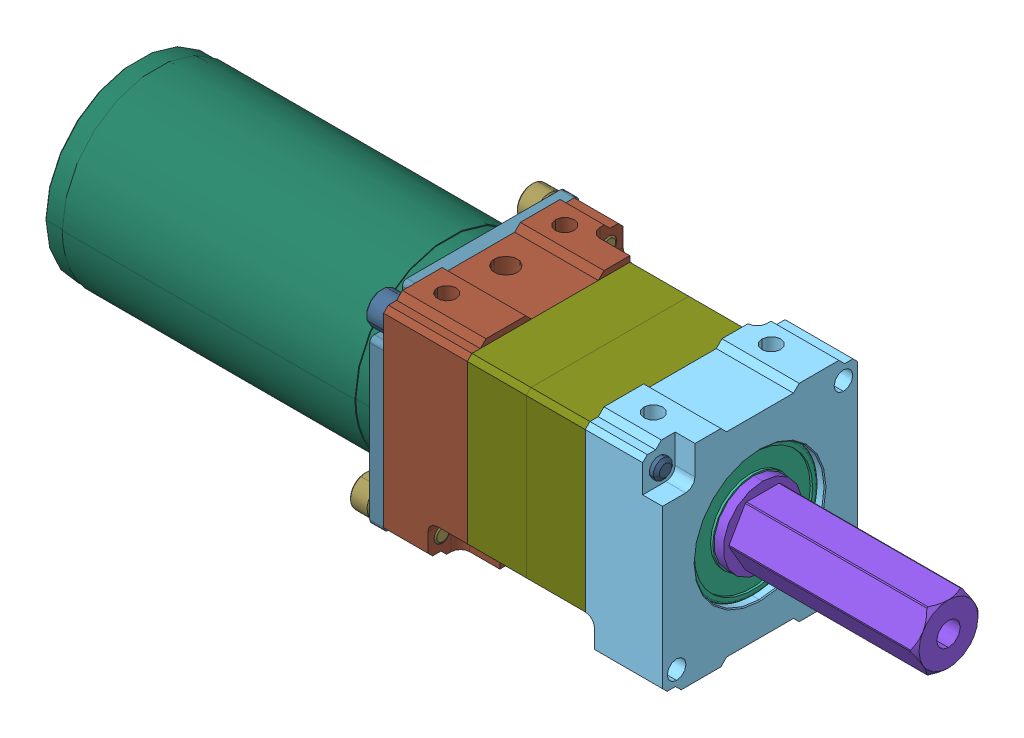
SolidWorks assembly VersaPlanetary v2 Two Stage 100 1 with BAG, configuration Default. Lengths in mm.
Overall size (176.1 63.52 63.52).
41 component instances, 19 part files, 0 mates.
Components (placement in the parent):
- VersaPlanetary v2 Two Stage 100 1 with BAG .step-1: VersaPlanetary v2 Two Stage 100 1 with BAG .step [Default] at origin size (176.1 63.52 63.52)
  - 217-2820 Rev1_Public.step-1: 217-2820 Rev1_Public.step [Default] at (-4.6546 22.225 0) x (0 -0.456494 0.889726) z (-1 0 0) size (39.22 38.88 17.4)
    - 217-2625-100.step-1: 217-2625-100.step [Default] at origin size (39.22 38.88 12.7)
      - 217-2625-008 Rev1.step-1: 217-2625-008 Rev1.step [Default] at origin size (34.7 34.7 4.7)
      - 217-2625-010 Rev1.step-1: 217-2625-010 Rev1.step [Default] at (0 10.193 3.65) x (0.999813 0.019336 0) z (0 0 1) size (4 4 12)
      - 217-2625-010 Rev1.step-2: 217-2625-010 Rev1.step [Default] at (8.691 -5.3258 3.65) size (4 4 12)
      - 217-2625-010 Rev1.step-3: 217-2625-010 Rev1.step [Default] at (-8.691 -5.3258 3.65) size (4 4 12)
      - 217-2625-005 Rev1_Planet_Revolving_Follower01.step-1: 217-2625-005 Rev1_Planet_Revolving_Follower01.step [Default] at (8.691 -5.3258 6.35) x (0.932816 0.360354 0) z (0 0 1) size (16.89 16.89 8)
      - 217-2625-005 Rev1_Planet_Revolving_Follower01.step-2: 217-2625-005 Rev1_Planet_Revolving_Follower01.step [Default] at (-8.691 -5.3258 6.35) x (-0.932788 -0.360426 0) z (0 0 1) size (16.89 16.89 8)
      - 217-2625-005 Rev1_Planet_Revolving_Follower01.step-3: 217-2625-005 Rev1_Planet_Revolving_Follower01.step [Default] at (0 10.193 6.35) x (0.893583 0.448898 0) z (0 0 1) size (16.89 16.89 8)
    - 217-2625-007 Rev1_Public.step-1: 217-2625-007 Rev1_Public.step [Default] at (0 0 6.7) x (0.992772 0.120019 0) z (0 0 1) size (15.27 15.27 12.7)
  - 217-2820 Rev1_Public.step-2: 217-2820 Rev1_Public.step [Default] at (-17.15 22.225 0) x (0 0.184082 0.982911) z (-1 0 0) size (39.22 38.88 17.4)
    - 217-2625-100.step-1: 217-2625-100.step [Default] at origin size (39.22 38.88 12.7)
      - 217-2625-008 Rev1.step-1: 217-2625-008 Rev1.step [Default] at origin size (34.7 34.7 4.7)
      - 217-2625-010 Rev1.step-1: 217-2625-010 Rev1.step [Default] at (0 10.193 3.65) x (0.999813 0.019336 0) z (0 0 1) size (4 4 12)
      - 217-2625-010 Rev1.step-2: 217-2625-010 Rev1.step [Default] at (8.691 -5.3258 3.65) size (4 4 12)
      - 217-2625-010 Rev1.step-3: 217-2625-010 Rev1.step [Default] at (-8.691 -5.3258 3.65) size (4 4 12)
      - 217-2625-005 Rev1_Planet_Revolving_Follower01.step-1: 217-2625-005 Rev1_Planet_Revolving_Follower01.step [Default] at (8.691 -5.3258 6.35) x (0.932816 0.360354 0) z (0 0 1) size (16.89 16.89 8)
      - 217-2625-005 Rev1_Planet_Revolving_Follower01.step-2: 217-2625-005 Rev1_Planet_Revolving_Follower01.step [Default] at (-8.691 -5.3258 6.35) x (-0.932788 -0.360426 0) z (0 0 1) size (16.89 16.89 8)
      - 217-2625-005 Rev1_Planet_Revolving_Follower01.step-3: 217-2625-005 Rev1_Planet_Revolving_Follower01.step [Default] at (0 10.193 6.35) x (0.893583 0.448898 0) z (0 0 1) size (16.89 16.89 8)
    - 217-2625-007 Rev1_Public.step-1: 217-2625-007 Rev1_Public.step [Default] at (0 0 6.7) x (0.992772 0.120019 0) z (0 0 1) size (15.27 15.27 12.7)
  - 217-2625-026 Rev1.step-1: 217-2625-026 Rev1.step [Default] at (-6.5 22.225 0) x (0 -1 0) z (-1 0 0) size (44.45 42 18.12)
  - 217-2742-001 Rev4.step-1: 217-2742-001 Rev4.step [Default] at (0.2002 22.225 0) x (1 0 0) z (0 -0.092627 0.995701) size (7 28 28)
  - 217-2742-001 Rev4.step-2: 217-2742-001 Rev4.step [Default] at (8.2002 22.225 0) size (7 28 28)
  - 217-2625-017 Rev1_9714K61.step-1: 217-2625-017 Rev1_9714K61.step [Default] at (7.42 22.3002 -0.342) x (0 0.56703 0.823697) z (0 -0.823697 0.56703) size (28.51 4.98 27.43)
  - 217-2625-003 Rev1.step-1: 217-2625-003 Rev1.step [Default] at (7.4478 22.225 0) x (0 -1 0) z (1 0 0) size (17 17 64.11)
  - 217-2625-018 Rev1_98541A410.step-1: 217-2625-018 Rev1_98541A410.step [Default] at (-0.7046 22.225 0) x (1 0 0) z (0 -0.017452 0.999848) size (1 19.6 17.4)
  - 832-2250-Base-Kit-Screw_SSA0832-0500ZC.step-1: 832-2250-Base-Kit-Screw_SSA0832-0500ZC.step [Default] at (-43.4 4.725 -17.5) x (0 -0.767799 -0.640691) z (0 0.640691 -0.767799) size (6.73 61.21 6.73)
  - 832-2250-Base-Kit-Screw_SSA0832-0500ZC.step-2: 832-2250-Base-Kit-Screw_SSA0832-0500ZC.step [Default] at (-43.4 39.725 17.5) x (0 0.961307 0.275478) z (0 -0.275478 0.961307) size (6.73 61.21 6.73)
  - 217-2625-025 Rev1.step-1: 217-2625-025 Rev1.step [Default] at (-35.9 22.225 0) x (0 -1 0) z (-1 0 0) size (44.45 42 18)
  - 217-4649-002 Rev1_SSA0832-0500ZC.step-1: 217-4649-002 Rev1_SSA0832-0500ZC.step [Default] at (-46.4 4.2645 17.9605) x (0 0.33842 -0.940995) z (0 0.940995 0.33842) size (6.73 16.76 6.73)
  - 217-4649-002 Rev1_SSA0832-0500ZC.step-2: 217-4649-002 Rev1_SSA0832-0500ZC.step [Default] at (-46.4 40.1855 -17.9605) x (0 -0.308932 -0.951084) z (0 0.951084 -0.308932) size (6.73 16.76 6.73)
  - 217-4649-006 Rev1_SSA0004-008BA.step-1: 217-4649-006 Rev1_SSA0004-008BA.step [Default] at (-43.4 22.225 12.5) x (0 0.5 -0.866025) z (0 -0.866025 -0.5) size (7 14 7)
  - 217-4649-006 Rev1_SSA0004-008BA.step-2: 217-4649-006 Rev1_SSA0004-008BA.step [Default] at (-43.4 22.225 -12.5) x (0 -0.5 0.866025) z (0 0.866025 0.5) size (7 14 7)
  - 217-2822-003 Rev4.step-1: 217-2822-003 Rev4.step [Default] at (-44.9 22.225 0) x (0 -1 0) z (-1 0 0) size (42 42 4.8)
  - 217-3351 Rev2.step-1: 217-3351 Rev2.step [Default] at (-46.4 22.225 0) x (0 0 1) z (1 0 0) size (59.07 59.07 84.5)
  - 217-2816-001 Rev1.step-1: 217-2816-001 Rev1.step [Default] at (-6.35 22.225 0) x (0 -1 0) z (1 0 0) size (42 42 14.51)
  - 217-2816-001 Rev1.step-2: 217-2816-001 Rev1.step [Default] at (-19.05 22.225 0) x (0 -1 0) z (1 0 0) size (42 42 14.51)
  - 217-4649-001 Rev1.step-1: 217-4649-001 Rev1.step [Default] at (-32.746 22.225 0) x (0 -1 0) z (1 0 0) size (18 18 13)
  - 217-4649-007 Rev1_94105A824.step-1: 217-4649-007 Rev1_94105A824.step [Default] at (-38.221 22.225 -6.7835) x (-0.996104 -0.088191 0) z (0 0 -1) size (4.83 4.83 4.77)
  - 217-2625-011 Rev1.step-1: 217-2625-011 Rev1.step [Default] at (-37.4818 22.225 0) x (0 0 1) z (0 -1 0) size (8.01 7.5 7.94)
